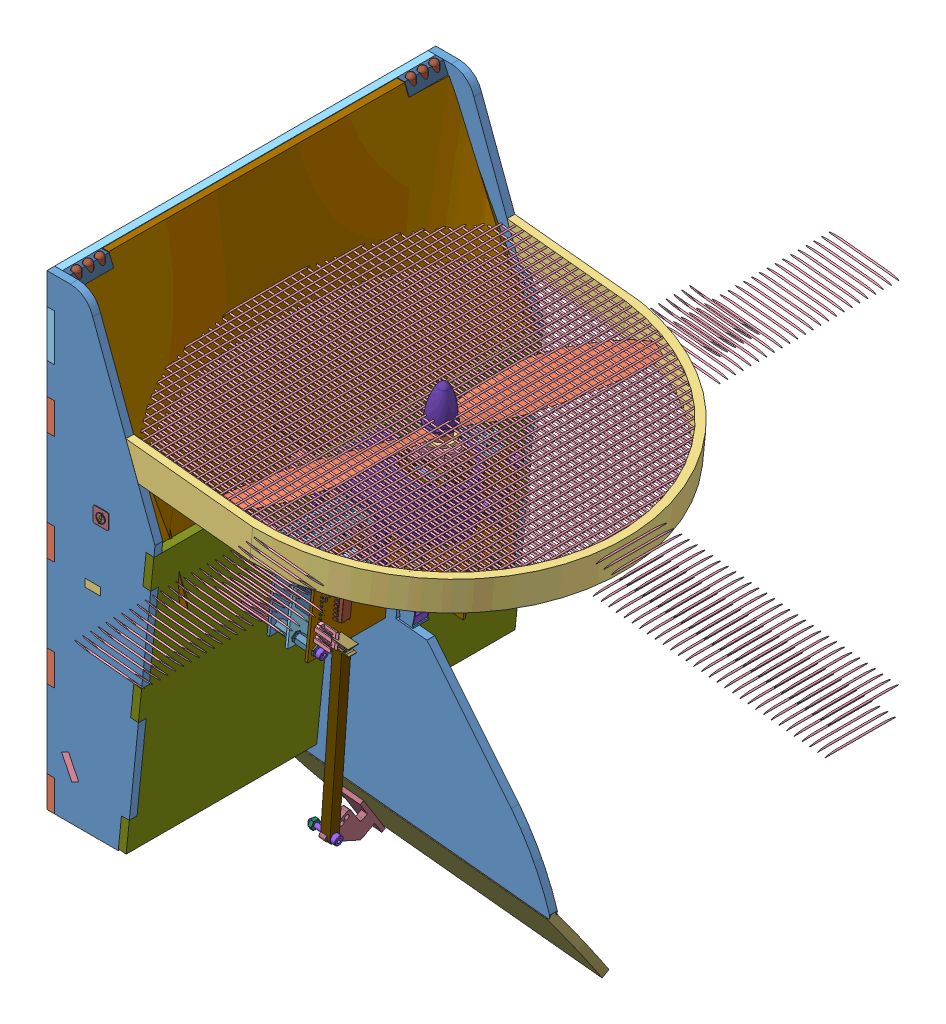
SolidWorks assembly AssTotaleSimu6, configuration Défaut. Lengths in mm. (continued)
Components (placement in the parent): (continued)
- AssStructSimu-1: AssStructSimu [Défaut] at (-125.7658 -1.8483 624.6548) x (1 0 0) z (0 0 -1) size (253.25 324.59 251.6) (continued)
  - AssCarte-1: AssCarte [Défaut] at (38.0121 147.1029 290.772) x (-0.101852 0.9948 0) z (0.9948 0.101852 0) size (66.52 130.57 98.72) (continued)
    - carte_onduleur_v3-1: carte_onduleur_v3 [Défaut] at (-131.8199 12.0892 20.7912) size (66.52 130.57 82.34) (continued)
      - RC2_2-1: RC2_2 [Défaut] at (-22 0.18 -0.803) x (-1 0 0) z (0 0 -1) size (2.34 1.04 0.5) (continued)
        - Open CASCADE STEP translator 6.8 1.12.1-1: Open CASCADE STEP translator 6.8 1.12.1 [Défaut] at origin size (2.34 1.04 0.5) (continued)
          - Pin_2_2-1: Pin_2_2 [Défaut] at origin size (0.51 1.02 0.5)
      - RC3_1-1: RC3_1 [Défaut] at (-20.9336 -14.5 -0.803) x (1 0 0) z (0 0 -1) size (2.34 1.04 0.5)
        - Open CASCADE STEP translator 6.8 1.12.1-1: Open CASCADE STEP translator 6.8 1.12.1 [Défaut] at origin size (2.34 1.04 0.5)
          - Body_1_3-1: Body_1_3 [Défaut] at origin size (2.29 1.04 0.43)
          - Pin_1_2-1: Pin_1_2 [Défaut] at (0.3048 0 0) x (-1 0 0) z (0 0 1) size (0.51 1.02 0.5)
          - Pin_2_2-1: Pin_2_2 [Défaut] at origin size (0.51 1.02 0.5)
      - RC3_2-1: RC3_2 [Défaut] at (-22.3 -14.5 -0.803) x (-1 0 0) z (0 0 -1) size (2.34 1.04 0.5)
        - Open CASCADE STEP translator 6.8 1.12.1-1: Open CASCADE STEP translator 6.8 1.12.1 [Défaut] at origin size (2.34 1.04 0.5)
          - Body_1_3-1: Body_1_3 [Défaut] at origin size (2.29 1.04 0.43)
          - Pin_1_2-1: Pin_1_2 [Défaut] at (0.3048 0 0) x (-1 0 0) z (0 0 1) size (0.51 1.02 0.5)
          - Pin_2_2-1: Pin_2_2 [Défaut] at origin size (0.51 1.02 0.5)
      - U_MES_CUR-1: U_MES_CUR [Défaut] at (-11.5 6.7816 0.803) size (2.54 2.41 0.76)
        - Open CASCADE STEP translator 6.8 1.32.1-1: Open CASCADE STEP translator 6.8 1.32.1 [Défaut] at origin size (2.54 2.41 0.76)
          - Body_1_5-1: Body_1_5 [Défaut] at origin size (2.54 1.27 0.71)
          - Pin_1_3-1: Pin_1_3 [Défaut] at (-2.1082 0.2286 0) x (0 -1 0) z (0 0 1) size (1.14 0.25 0.47)
          - Pin_2_3-1: Pin_2_3 [Défaut] at (-0.2032 2.1336 0) x (0 -1 0) z (0 0 1) size (1.14 0.25 0.47)
      - CARTE_ALIM-1: CARTE_ALIM [Défaut] at (-6.4 -57.2 0.803) size (60 130 18.35)
        - Open CASCADE STEP translator 6.8 1.33.1-1: Open CASCADE STEP translator 6.8 1.33.1 [Défaut] at origin size (60 130 18.35)
          - Body_1_6-1: Body_1_6 [Défaut] at (7 56 -12) size (60 130 18.35)
            - 1_3-1: 1_3 [Défaut] at origin size (60 130 1.61)
            - 13_3-1: 13_3 [Défaut] at (0.4717 -40.93 0.803) x (0 1 0) z (0 0 1) size (5.65 4.9 1.7)
              - =_[0_1_1_4]_3-1: =_[0_1_1_4]_3 [Défaut] at origin size (5.65 4.9 1.7)
                - 2-1: 2 [Défaut] at origin size (3.75 4.9 1.53)
                - 3-1: 3 [Défaut] at origin size (0.95 0.51 1.06)
                - 4-1: 4 [Défaut] at origin size (0.95 0.51 1.06)
                - 5_2-1: 5_2 [Défaut] at origin size (0.95 0.51 1.06)
                - 6-1: 6 [Défaut] at origin size (0.95 0.51 1.06)
                - 7-1: 7 [Défaut] at (10.8 -5.08 0) x (-1 0 0) z (0 0 1) size (0.95 0.51 1.06)
                - 8_2-1: 8_2 [Défaut] at (10.8 -2.54 0) x (-1 0 0) z (0 0 1) size (0.95 0.51 1.06)
                - 9-1: 9 [Défaut] at (10.8 0 0) x (-1 0 0) z (0 0 1) size (0.95 0.51 1.06)
                - 10-1: 10 [Défaut] at (10.8 2.54 0) x (-1 0 0) z (0 0 1) size (0.95 0.51 1.06)
                - 11_2-1: 11_2 [Défaut] at (5.4 -1.27 0) x (-1 0 0) z (0 0 1) size (4.25 2.34 1.06)
            - 18-1: 18 [Défaut] at (-2.5283 -37.23 0.803) x (0 -1 0) z (0 0 1) size (2.34 1.04 0.5)
              - =_[0_1_1_16]-1: =_[0_1_1_16] [Défaut] at origin size (2.34 1.04 0.5)
                - 14_2-1: 14_2 [Défaut] at origin size (2.29 1.04 0.43)
                - 15_2-1: 15_2 [Défaut] at (0.3048 0 0) x (-1 0 0) z (0 0 1) size (0.51 1.02 0.5)
                - 16_2-1: 16_2 [Défaut] at origin size (0.51 1.02 0.5)
            - 21_2-1: 21_2 [Défaut] at (-2.2263 -24.628 -0.803) x (1 0 0) z (0 0 -1) size (8.01 8 14.24)
              - =_[0_1_1_21]-1: =_[0_1_1_21] [Défaut] at origin size (8.01 8 14.24)
                - 19-1: 19 [Défaut] at (1.8 0 0) x (1 0 0) z (0 -1 0) size (8.01 14.24 8)
            - 23_2-1: 23_2 [Défaut] at (1.2381 -31.53 0.803) size (2.34 1.04 0.5)
              - =_[0_1_1_16]-1: =_[0_1_1_16] [Défaut] at origin size (2.34 1.04 0.5)
                - 14_2-1: 14_2 [Défaut] at origin size (2.29 1.04 0.43)
                - 15_2-1: 15_2 [Défaut] at (0.3048 0 0) x (-1 0 0) z (0 0 1) size (0.51 1.02 0.5)
                - 16_2-1: 16_2 [Défaut] at origin size (0.51 1.02 0.5)
            - 28-1: 28 [Défaut] at (5 29.8636 0.803) x (0 -1 0) z (0 0 1) size (3.35 1.3 0.55)
              - =_[0_1_1_25]_2-1: =_[0_1_1_25]_2 [Défaut] at origin size (3.35 1.3 0.55)
                - 24-1: 24 [Défaut] at origin size (3.3 1.3 0.48)
                - 25_2-1: 25_2 [Défaut] at (0.5588 0 0) x (-1 0 0) z (0 0 1) size (0.76 1.27 0.55)
                - 26_2-1: 26_2 [Défaut] at origin size (0.76 1.27 0.55)
            - 30-1: 30 [Défaut] at (6.7 29.8636 0.803) x (0 -1 0) z (0 0 1) size (2.34 1.04 0.5)
              - =_[0_1_1_16]-1: =_[0_1_1_16] [Défaut] at origin size (2.34 1.04 0.5)
                - 14_2-1: 14_2 [Défaut] at origin size (2.29 1.04 0.43)
                - 15_2-1: 15_2 [Défaut] at (0.3048 0 0) x (-1 0 0) z (0 0 1) size (0.51 1.02 0.5)
                - 16_2-1: 16_2 [Défaut] at origin size (0.51 1.02 0.5)
            - 35_2-1: 35_2 [Défaut] at (-2.5 -46.37 0.803) x (0 1 0) z (0 0 1) size (3.4 2.06 0.79)
              - =_[0_1_1_31]-1: =_[0_1_1_31] [Défaut] at origin size (3.4 2.06 0.79)
                - 31_2-1: 31_2 [Défaut] at origin size (3.3 2.06 0.69)
                - 32_3-1: 32_3 [Défaut] at (0.5588 0 0) x (-1 0 0) z (0 0 1) size (0.81 2.03 0.79)
                - 33_3-1: 33_3 [Défaut] at origin size (0.81 2.03 0.79)
            - 37-1: 37 [Défaut] at (5 31.43 0.803) x (0 1 0) z (0 0 1) size (2.34 1.04 0.5)
              - =_[0_1_1_16]-1: =_[0_1_1_16] [Défaut] at origin size (2.34 1.04 0.5)
                - 14_2-1: 14_2 [Défaut] at origin size (2.29 1.04 0.43)
                - 15_2-1: 15_2 [Défaut] at (0.3048 0 0) x (-1 0 0) z (0 0 1) size (0.51 1.02 0.5)
                - 16_2-1: 16_2 [Défaut] at origin size (0.51 1.02 0.5)
            - 39-1: 39 [Défaut] at (-0.2 35.63 0.803) x (-1 0 0) z (0 0 1) size (2.34 1.04 0.5)
              - =_[0_1_1_16]-1: =_[0_1_1_16] [Défaut] at origin size (2.34 1.04 0.5)
                - 14_2-1: 14_2 [Défaut] at origin size (2.29 1.04 0.43)
                - 15_2-1: 15_2 [Défaut] at (0.3048 0 0) x (-1 0 0) z (0 0 1) size (0.51 1.02 0.5)
                - 16_2-1: 16_2 [Défaut] at origin size (0.51 1.02 0.5)
            - 41-1: 41 [Défaut] at (2.9 -45.5036 0.803) x (0 1 0) z (0 0 1) size (2.34 1.04 0.5)
              - =_[0_1_1_16]-1: =_[0_1_1_16] [Défaut] at origin size (2.34 1.04 0.5)
                - 14_2-1: 14_2 [Défaut] at origin size (2.29 1.04 0.43)
                - 15_2-1: 15_2 [Défaut] at (0.3048 0 0) x (-1 0 0) z (0 0 1) size (0.51 1.02 0.5)
                - 16_2-1: 16_2 [Défaut] at origin size (0.51 1.02 0.5)
            - 43-1: 43 [Défaut] at (17.1348 -42.6272 0.803) x (0 1 0) z (0 0 1) size (2.34 1.04 0.5)
              - =_[0_1_1_16]-1: =_[0_1_1_16] [Défaut] at origin size (2.34 1.04 0.5)
                - 14_2-1: 14_2 [Défaut] at origin size (2.29 1.04 0.43)
                - 15_2-1: 15_2 [Défaut] at (0.3048 0 0) x (-1 0 0) z (0 0 1) size (0.51 1.02 0.5)
                - 16_2-1: 16_2 [Défaut] at origin size (0.51 1.02 0.5)
            - 48_2-1: 48_2 [Défaut] at (-5.4717 -39.01 0.803) x (-1 0 0) z (0 0 1) size (4.19 3.4 1.75)
              - =_[0_1_1_40]-1: =_[0_1_1_40] [Défaut] at origin size (4.19 3.4 1.75)
                - 44_2-1: 44_2 [Défaut] at origin size (3.75 3.38 1.73)
                - 45_2-1: 45_2 [Défaut] at (0.438 0 0) x (-1 0 0) z (0 0 1) size (0.53 3.4 1.75)
                - 46_2-1: 46_2 [Défaut] at origin size (0.52 3.4 1.75)
            - 53-1: 53 [Défaut] at (0.9 35.63 0.803) size (2.34 1.04 0.5)
              - =_[0_1_1_45]-1: =_[0_1_1_45] [Défaut] at origin size (2.34 1.04 0.5)
                - 49_3-1: 49_3 [Défaut] at origin size (2.29 1.04 0.43)
                - 50-1: 50 [Défaut] at (0.3048 0 0) x (-1 0 0) z (0 0 1) size (0.51 1.02 0.5)
                - 51-1: 51 [Défaut] at origin size (0.51 1.02 0.5)
            - 55_2-1: 55_2 [Défaut] at (1.3 -45.5036 0.803) x (0 1 0) z (0 0 1) size (2.34 1.04 0.5)
              - =_[0_1_1_45]-1: =_[0_1_1_45] [Défaut] at origin size (2.34 1.04 0.5)
                - 49_3-1: 49_3 [Défaut] at origin size (2.29 1.04 0.43)
                - 50-1: 50 [Défaut] at (0.3048 0 0) x (-1 0 0) z (0 0 1) size (0.51 1.02 0.5)
                - 51-1: 51 [Défaut] at origin size (0.51 1.02 0.5)
            - 57_3-1: 57_3 [Défaut] at (17.2348 -43.9936 0.803) x (0 -1 0) z (0 0 1) size (2.34 1.04 0.5)
              - =_[0_1_1_45]-1: =_[0_1_1_45] [Défaut] at origin size (2.34 1.04 0.5)
                - 49_3-1: 49_3 [Défaut] at origin size (2.29 1.04 0.43)
                - 50-1: 50 [Défaut] at (0.3048 0 0) x (-1 0 0) z (0 0 1) size (0.51 1.02 0.5)
                - 51-1: 51 [Défaut] at origin size (0.51 1.02 0.5)
            - 65-1: 65 [Défaut] at (-4.8 30.93 0.803) x (-1 0 0) z (0 0 1) size (14.64 9.83 4.25)
              - =_[0_1_1_52]-1: =_[0_1_1_52] [Défaut] at origin size (14.64 9.83 4.25)
                - 63_2-1: 63_2 [Défaut] at (3 0 0) x (0 -1 0) z (0 0 1) size (9.83 14.64 4.25)
                  - =_[0_1_1_3]_5-1: =_[0_1_1_3]_5 [Défaut] at origin size (9.83 9.05 4.21)
                  - =_[0_1_1_4]_5-1: =_[0_1_1_4]_5 [Défaut] at origin size (9.48 7.76 1.21)
                  - =_[0_1_1_5]_5-1: =_[0_1_1_5]_5 [Défaut] at origin size (1.36 6.01 3.08)
                  - =_[0_1_1_6]_3-1: =_[0_1_1_6]_3 [Défaut] at origin size (1.36 6.01 3.08)
                  - =_[0_1_1_7]_3-1: =_[0_1_1_7]_3 [Défaut] at origin size (1.06 6.01 3.08)
            - 67-1: 67 [Défaut] at (13.5933 -37.5272 0.803) x (-1 0 0) z (0 0 1) size (2.34 1.04 0.5)
              - =_[0_1_1_16]-1: =_[0_1_1_16] [Défaut] at origin size (2.34 1.04 0.5)
                - 14_2-1: 14_2 [Défaut] at origin size (2.29 1.04 0.43)
                - 15_2-1: 15_2 [Défaut] at (0.3048 0 0) x (-1 0 0) z (0 0 1) size (0.51 1.02 0.5)
                - 16_2-1: 16_2 [Défaut] at origin size (0.51 1.02 0.5)
            - 70_2-1: 70_2 [Défaut] at (18.2733 -29.7272 0.803) x (0 1 0) z (0 0 1) size (6.06 4.95 1.88)
              - =_[0_1_1_61]-1: =_[0_1_1_61] [Défaut] at origin size (6.06 4.95 1.88)
                - 68-1: 68 [Défaut] x (1 0 0) z (0 -1 0) size (6.06 1.88 4.95)
            - 83-1: 83 [Défaut] at (-21.2 -38.07 0.803) x (-1 0 0) z (0 0 1) size (2.7 5.2 1.11)
              - =_[0_1_1_64]-1: =_[0_1_1_64] [Défaut] at origin size (2.7 5.2 1.11)
                - 84_2-1: 84_2 [Défaut] at (1.2 -4 0) x (0 1 0) z (0 0 1) size (5.2 2.7 1.11)
                  - =_[0_1_1_3]_6-1: =_[0_1_1_3]_6 [Défaut] at origin size (0.39 0.64 0.01)
                  - =_[0_1_1_4]_6-1: =_[0_1_1_4]_6 [Défaut] at origin size (0.6 1.9 0.2)
                  - =_[0_1_1_5]_6-1: =_[0_1_1_5]_6 [Défaut] at origin size (0.21 0.08 0.01)
                  - =_[0_1_1_6]_4-1: =_[0_1_1_6]_4 [Défaut] at origin size (0.6 1.9 0.2)
                  - =_[0_1_1_7]_4-1: =_[0_1_1_7]_4 [Défaut] at origin size (0.46 0.68 0.01)
                  - =_[0_1_1_8]_3-1: =_[0_1_1_8]_3 [Défaut] at origin size (0.38 0.66 0.01)
                  - =_[0_1_1_9]_2-1: =_[0_1_1_9]_2 [Défaut] at origin size (0.2 0.62 0.01)
                  - =_[0_1_1_10]_2-1: =_[0_1_1_10]_2 [Défaut] at origin size (4 2.7 1.1)
                  - =_[0_1_1_11]_2-1: =_[0_1_1_11]_2 [Défaut] at origin size (0.46 0.63 0.01)
                  - =_[0_1_1_12]_2-1: =_[0_1_1_12]_2 [Défaut] at origin size (0.56 0.68 0.01)
            - 86_2-1: 86_2 [Défaut] at (12.8933 -35.4272 0.803) x (0 1 0) z (0 0 1) size (2.7 5.2 1.11)
              - =_[0_1_1_77]-1: =_[0_1_1_77] [Défaut] at origin size (2.7 5.2 1.11)
                - 84_2-1: 84_2 [Défaut] at (1.2 -4 0) x (0 1 0) z (0 0 1) size (5.2 2.7 1.11)
                  - =_[0_1_1_3]_6-1: =_[0_1_1_3]_6 [Défaut] at origin size (0.39 0.64 0.01)
                  - =_[0_1_1_4]_6-1: =_[0_1_1_4]_6 [Défaut] at origin size (0.6 1.9 0.2)
                  - =_[0_1_1_5]_6-1: =_[0_1_1_5]_6 [Défaut] at origin size (0.21 0.08 0.01)
                  - =_[0_1_1_6]_4-1: =_[0_1_1_6]_4 [Défaut] at origin size (0.6 1.9 0.2)
                  - =_[0_1_1_7]_4-1: =_[0_1_1_7]_4 [Défaut] at origin size (0.46 0.68 0.01)
                  - =_[0_1_1_8]_3-1: =_[0_1_1_8]_3 [Défaut] at origin size (0.38 0.66 0.01)
                  - =_[0_1_1_9]_2-1: =_[0_1_1_9]_2 [Défaut] at origin size (0.2 0.62 0.01)
                  - =_[0_1_1_10]_2-1: =_[0_1_1_10]_2 [Défaut] at origin size (4 2.7 1.1)
                  - =_[0_1_1_11]_2-1: =_[0_1_1_11]_2 [Défaut] at origin size (0.46 0.63 0.01)
                  - =_[0_1_1_12]_2-1: =_[0_1_1_12]_2 [Défaut] at origin size (0.56 0.68 0.01)
            - 92_2-1: 92_2 [Défaut] at (20.9933 -39.3272 0.803) x (0 -1 0) z (0 0 1) size (2.79 1.98 0.64)
              - =_[0_1_1_79]-1: =_[0_1_1_79] [Défaut] at origin size (2.79 1.98 0.64)
                - 87-1: 87 [Défaut] at origin size (2.79 1.02 0.58)
                - 88-1: 88 [Défaut] x (0 -1 0) z (0 0 1) size (0.42 0.38 0.38)
                - 89-1: 89 [Défaut] at (-2.8448 -0.9652 0) x (0 1 0) z (0 0 1) size (0.55 0.38 0.38)
                - 90-1: 90 [Défaut] at (-0.9652 -2.8448 0) x (0 1 0) z (0 0 1) size (0.55 0.38 0.38)
            - 98-1: 98 [Défaut] at (-17.7 -48.47 0.803) x (0 -1 0) z (0 0 1) size (2.54 1.98 0.64)
              - =_[0_1_1_85]-1: =_[0_1_1_85] [Défaut] at origin size (2.54 1.98 0.64)
                - 93-1: 93 [Défaut] at origin size (2.54 1.14 0.58)
                - 94-1: 94 [Défaut] x (0 -1 0) z (0 0 1) size (0.43 0.51 0.38)
                - 95-1: 95 [Défaut] at (1.8796 1.8796 0) x (0 -1 0) z (0 0 1) size (0.43 0.51 0.38)
                - 96-1: 96 [Défaut] at (-0.9652 -2.8448 0) x (0 1 0) z (0 0 1) size (0.41 0.51 0.38)
            - 100-1: 100 [Défaut] at (24.3933 -43.2272 0.803) size (2.79 1.98 0.64)
              - =_[0_1_1_79]-1: =_[0_1_1_79] [Défaut] at origin size (2.79 1.98 0.64)
                - 87-1: 87 [Défaut] at origin size (2.79 1.02 0.58)
                - 88-1: 88 [Défaut] x (0 -1 0) z (0 0 1) size (0.42 0.38 0.38)
                - 89-1: 89 [Défaut] at (-2.8448 -0.9652 0) x (0 1 0) z (0 0 1) size (0.55 0.38 0.38)
                - 90-1: 90 [Défaut] at (-0.9652 -2.8448 0) x (0 1 0) z (0 0 1) size (0.55 0.38 0.38)
            - 102-1: 102 [Défaut] at (21.4933 -44.4272 0.803) x (0 -1 0) z (0 0 1) size (2.79 1.98 0.64)
              - =_[0_1_1_79]-1: =_[0_1_1_79] [Défaut] at origin size (2.79 1.98 0.64)
                - 87-1: 87 [Défaut] at origin size (2.79 1.02 0.58)
                - 88-1: 88 [Défaut] x (0 -1 0) z (0 0 1) size (0.42 0.38 0.38)
                - 89-1: 89 [Défaut] at (-2.8448 -0.9652 0) x (0 1 0) z (0 0 1) size (0.55 0.38 0.38)
                - 90-1: 90 [Défaut] at (-0.9652 -2.8448 0) x (0 1 0) z (0 0 1) size (0.55 0.38 0.38)
            - 107-1: 107 [Défaut] at (23.1933 -29.1272 -0.803) x (0 1 0) z (0 0 -1) size (9.6 14.35 5)
              - =_[0_1_1_93]-1: =_[0_1_1_93] [Défaut] at origin size (9.6 14.35 5)
                - 105-1: 105 [Défaut] at (0.5 -1 2) x (-1 0 0) z (0 0 1) size (9.6 14.35 5)
                  - =_[0_1_1_3]_7-1: =_[0_1_1_3]_7 [Défaut] at origin size (9.6 12.75 5)
                  - =_[0_1_1_4]_7-1: =_[0_1_1_4]_7 [Défaut] at origin size (2.2 1.6 2.2)
            - 109-1: 109 [Défaut] at (25.4933 -41.1272 0.803) x (-1 0 0) z (0 0 1) size (2.34 1.04 0.5)
              - =_[0_1_1_45]-1: =_[0_1_1_45] [Défaut] at origin size (2.34 1.04 0.5)
                - 49_3-1: 49_3 [Défaut] at origin size (2.29 1.04 0.43)
                - 50-1: 50 [Défaut] at (0.3048 0 0) x (-1 0 0) z (0 0 1) size (0.51 1.02 0.5)
                - 51-1: 51 [Défaut] at origin size (0.51 1.02 0.5)
            - 111-1: 111 [Défaut] at (22.0269 -41.8272 0.803) x (-1 0 0) z (0 0 1) size (2.34 1.04 0.5)
              - =_[0_1_1_45]-1: =_[0_1_1_45] [Défaut] at origin size (2.34 1.04 0.5)
                - 49_3-1: 49_3 [Défaut] at origin size (2.29 1.04 0.43)
                - 50-1: 50 [Défaut] at (0.3048 0 0) x (-1 0 0) z (0 0 1) size (0.51 1.02 0.5)
                - 51-1: 51 [Défaut] at origin size (0.51 1.02 0.5)
            - 113-1: 113 [Défaut] at (-24.8 -36.7036 0.803) x (0 1 0) z (0 0 1) size (2.34 1.04 0.5)
              - =_[0_1_1_45]-1: =_[0_1_1_45] [Défaut] at origin size (2.34 1.04 0.5)
                - 49_3-1: 49_3 [Défaut] at origin size (2.29 1.04 0.43)
                - 50-1: 50 [Défaut] at (0.3048 0 0) x (-1 0 0) z (0 0 1) size (0.51 1.02 0.5)
                - 51-1: 51 [Défaut] at origin size (0.51 1.02 0.5)
            - 115-1: 115 [Défaut] at (-24.8 -40.3036 0.803) x (0 1 0) z (0 0 1) size (2.34 1.04 0.5)
              - =_[0_1_1_45]-1: =_[0_1_1_45] [Défaut] at origin size (2.34 1.04 0.5)
                - 49_3-1: 49_3 [Défaut] at origin size (2.29 1.04 0.43)
                - 50-1: 50 [Défaut] at (0.3048 0 0) x (-1 0 0) z (0 0 1) size (0.51 1.02 0.5)
                - 51-1: 51 [Défaut] at origin size (0.51 1.02 0.5)
            - 117-1: 117 [Défaut] at (-16 -48.27 0.803) x (0 -1 0) z (0 0 1) size (2.34 1.04 0.5)
              - =_[0_1_1_45]-1: =_[0_1_1_45] [Défaut] at origin size (2.34 1.04 0.5)
                - 49_3-1: 49_3 [Défaut] at origin size (2.29 1.04 0.43)
                - 50-1: 50 [Défaut] at (0.3048 0 0) x (-1 0 0) z (0 0 1) size (0.51 1.02 0.5)
                - 51-1: 51 [Défaut] at origin size (0.51 1.02 0.5)
            - 119-1: 119 [Défaut] at (-22.5189 -47.87 0.803) x (-1 0 0) z (0 0 1) size (2.34 1.04 0.5)
              - =_[0_1_1_45]-1: =_[0_1_1_45] [Défaut] at origin size (2.34 1.04 0.5)
                - 49_3-1: 49_3 [Défaut] at origin size (2.29 1.04 0.43)
                - 50-1: 50 [Défaut] at (0.3048 0 0) x (-1 0 0) z (0 0 1) size (0.51 1.02 0.5)
                - 51-1: 51 [Défaut] at origin size (0.51 1.02 0.5)
            - 121-1: 121 [Défaut] at (22.3933 -38.9272 0.803) size (2.34 1.04 0.5)
              - =_[0_1_1_45]-1: =_[0_1_1_45] [Défaut] at origin size (2.34 1.04 0.5)
                - 49_3-1: 49_3 [Défaut] at origin size (2.29 1.04 0.43)
                - 50-1: 50 [Défaut] at (0.3048 0 0) x (-1 0 0) z (0 0 1) size (0.51 1.02 0.5)
                - 51-1: 51 [Défaut] at origin size (0.51 1.02 0.5)
            - 123-1: 123 [Défaut] at (22.0933 -36.4272 0.803) x (-1 0 0) z (0 0 1) size (2.34 1.04 0.5)
              - =_[0_1_1_45]-1: =_[0_1_1_45] [Défaut] at origin size (2.34 1.04 0.5)
                - 49_3-1: 49_3 [Défaut] at origin size (2.29 1.04 0.43)
                - 50-1: 50 [Défaut] at (0.3048 0 0) x (-1 0 0) z (0 0 1) size (0.51 1.02 0.5)
                - 51-1: 51 [Défaut] at origin size (0.51 1.02 0.5)
            - 125-1: 125 [Défaut] at (22.3933 -32.0272 0.803) x (0 -1 0) z (0 0 1) size (2.34 1.04 0.5)
              - =_[0_1_1_45]-1: =_[0_1_1_45] [Défaut] at origin size (2.34 1.04 0.5)
                - 49_3-1: 49_3 [Défaut] at origin size (2.29 1.04 0.43)
                - 50-1: 50 [Défaut] at (0.3048 0 0) x (-1 0 0) z (0 0 1) size (0.51 1.02 0.5)
                - 51-1: 51 [Défaut] at origin size (0.51 1.02 0.5)
            - 127-1: 127 [Défaut] at (17.9597 -23.1272 0.803) size (2.34 1.04 0.5)
              - =_[0_1_1_16]-1: =_[0_1_1_16] [Défaut] at origin size (2.34 1.04 0.5)
                - 14_2-1: 14_2 [Défaut] at origin size (2.29 1.04 0.43)
                - 15_2-1: 15_2 [Défaut] at (0.3048 0 0) x (-1 0 0) z (0 0 1) size (0.51 1.02 0.5)
                - 16_2-1: 16_2 [Défaut] at origin size (0.51 1.02 0.5)
            - 129-1: 129 [Défaut] at (20.0269 -24.9272 0.803) x (-1 0 0) z (0 0 1) size (2.34 1.04 0.5)
              - =_[0_1_1_16]-1: =_[0_1_1_16] [Défaut] at origin size (2.34 1.04 0.5)
                - 14_2-1: 14_2 [Défaut] at origin size (2.29 1.04 0.43)
                - 15_2-1: 15_2 [Défaut] at (0.3048 0 0) x (-1 0 0) z (0 0 1) size (0.51 1.02 0.5)
                - 16_2-1: 16_2 [Défaut] at origin size (0.51 1.02 0.5)
            - 131-1: 131 [Défaut] at (16.9933 -37.5272 0.803) x (-1 0 0) z (0 0 1) size (2.34 1.04 0.5)
              - =_[0_1_1_45]-1: =_[0_1_1_45] [Défaut] at origin size (2.34 1.04 0.5)
                - 49_3-1: 49_3 [Défaut] at origin size (2.29 1.04 0.43)
                - 50-1: 50 [Défaut] at (0.3048 0 0) x (-1 0 0) z (0 0 1) size (0.51 1.02 0.5)
                - 51-1: 51 [Défaut] at origin size (0.51 1.02 0.5)
            - 136-1: 136 [Défaut] at (3.2957 -29.23 0.803) x (-1 0 0) z (0 0 1) size (4.78 2.79 2.03)
              - =_[0_1_1_110]_2-1: =_[0_1_1_110]_2 [Défaut] at origin size (4.78 2.79 2.03)
                - 132-1: 132 [Défaut] at origin size (4.32 2.79 1.78)
                - 133-1: 133 [Défaut] at (0.4572 0 0) x (-1 0 0) z (0 0 1) size (1.02 1.27 1.32)
                - 134-1: 134 [Défaut] at origin size (1.02 1.27 1.32)
            - 141-1: 141 [Défaut] at (0.2436 -33.3673 0.803) size (3.35 1.3 0.55)
              - =_[0_1_1_115]_2-1: =_[0_1_1_115]_2 [Défaut] at origin size (3.35 1.3 0.55)
                - 137-1: 137 [Défaut] at origin size (3.3 1.3 0.48)
                - 138-1: 138 [Défaut] at (0.5588 0 0) x (-1 0 0) z (0 0 1) size (0.76 1.27 0.55)
                - 139-1: 139 [Défaut] at origin size (0.76 1.27 0.55)
            - 143_2-1: 143_2 [Défaut] at (-0.3 -45.47 0.803) x (0 1 0) z (0 0 1) size (2.34 1.04 0.5)
              - =_[0_1_1_16]-1: =_[0_1_1_16] [Défaut] at origin size (2.34 1.04 0.5)
                - 14_2-1: 14_2 [Défaut] at origin size (2.29 1.04 0.43)
                - 15_2-1: 15_2 [Défaut] at (0.3048 0 0) x (-1 0 0) z (0 0 1) size (0.51 1.02 0.5)
                - 16_2-1: 16_2 [Défaut] at origin size (0.51 1.02 0.5)
            - 145-1: 145 [Défaut] at (6.6 31.13 0.803) x (0 1 0) z (0 0 1) size (3.35 1.3 0.55)
              - =_[0_1_1_25]_2-1: =_[0_1_1_25]_2 [Défaut] at origin size (3.35 1.3 0.55)
                - 24-1: 24 [Défaut] at origin size (3.3 1.3 0.48)
                - 25_2-1: 25_2 [Défaut] at (0.5588 0 0) x (-1 0 0) z (0 0 1) size (0.76 1.27 0.55)
                - 26_2-1: 26_2 [Défaut] at origin size (0.76 1.27 0.55)
            - 148-1: 148 [Défaut] at (-7.5 -56.57 0.803) size (15.24 2.54 7.37)
              - =_[0_1_1_122]_2-1: =_[0_1_1_122]_2 [Défaut] at origin size (15.24 2.54 7.37)
                - 146-1: 146 [Défaut] at (6.3 0 1) x (1 0 0) z (0 -1 0) size (15.24 7.37 2.54)
      - COMP1-1: COMP1 [Défaut] at (-16.3 -36.2 0.803) x (-1 0 0) z (0 0 1) size (2.03 1.88 0.51)
        - Open CASCADE STEP translator 6.8 1.34.1-1: Open CASCADE STEP translator 6.8 1.34.1 [Défaut] at origin size (2.03 1.88 0.51)
          - Body_1_6-1: Body_1_6 [Défaut] at origin size (2.03 1.02 0.46)
          - Pin_1_4-1: Pin_1_4 [Défaut] x (0 1 0) z (0 0 1) size (0.45 0.25 0.32)
          - Pin_2_4-1: Pin_2_4 [Défaut] at (0.65 -0.65 0) x (0 1 0) z (0 0 1) size (0.45 0.25 0.32)
          - Pin_3-1: Pin_3 [Défaut] at (1.3 -1.3 0) x (0 1 0) z (0 0 1) size (0.45 0.25 0.32)
          - Pin_4-1: Pin_4 [Défaut] at (-0.5 3.1 0) x (0 -1 0) z (0 0 1) size (0.41 0.25 0.32)
          - Pin_5-1: Pin_5 [Défaut] at (-1.8 1.8 0) x (0 -1 0) z (0 0 1) size (0.41 0.25 0.32)
      - COMP2-1: COMP2 [Défaut] at (-14.3 -9.6 0.803) x (-1 0 0) z (0 0 1) size (2.03 1.88 0.51)
        - Open CASCADE STEP translator 6.8 1.34.1-1: Open CASCADE STEP translator 6.8 1.34.1 [Défaut] at origin size (2.03 1.88 0.51)
          - Body_1_6-1: Body_1_6 [Défaut] at origin size (2.03 1.02 0.46)
          - Pin_1_4-1: Pin_1_4 [Défaut] x (0 1 0) z (0 0 1) size (0.45 0.25 0.32)
          - Pin_2_4-1: Pin_2_4 [Défaut] at (0.65 -0.65 0) x (0 1 0) z (0 0 1) size (0.45 0.25 0.32)
          - Pin_3-1: Pin_3 [Défaut] at (1.3 -1.3 0) x (0 1 0) z (0 0 1) size (0.45 0.25 0.32)
          - Pin_4-1: Pin_4 [Défaut] at (-0.5 3.1 0) x (0 -1 0) z (0 0 1) size (0.41 0.25 0.32)
          - Pin_5-1: Pin_5 [Défaut] at (-1.8 1.8 0) x (0 -1 0) z (0 0 1) size (0.41 0.25 0.32)
      - COMP3-1: COMP3 [Défaut] at (-15.9 -23.2 0.803) x (-1 0 0) z (0 0 1) size (2.03 1.88 0.51)
        - Open CASCADE STEP translator 6.8 1.34.1-1: Open CASCADE STEP translator 6.8 1.34.1 [Défaut] at origin size (2.03 1.88 0.51)
          - Body_1_6-1: Body_1_6 [Défaut] at origin size (2.03 1.02 0.46)
          - Pin_1_4-1: Pin_1_4 [Défaut] x (0 1 0) z (0 0 1) size (0.45 0.25 0.32)
          - Pin_2_4-1: Pin_2_4 [Défaut] at (0.65 -0.65 0) x (0 1 0) z (0 0 1) size (0.45 0.25 0.32)
          - Pin_3-1: Pin_3 [Défaut] at (1.3 -1.3 0) x (0 1 0) z (0 0 1) size (0.45 0.25 0.32)
          - Pin_4-1: Pin_4 [Défaut] at (-0.5 3.1 0) x (0 -1 0) z (0 0 1) size (0.41 0.25 0.32)
          - Pin_5-1: Pin_5 [Défaut] at (-1.8 1.8 0) x (0 -1 0) z (0 0 1) size (0.41 0.25 0.32)
      - CP1-1: CP1 [Défaut] at (-18.9 -38.2 0.803) x (0 1 0) z (0 0 1) size (2.34 1.04 0.5)
        - Open CASCADE STEP translator 6.8 1.6.1-1: Open CASCADE STEP translator 6.8 1.6.1 [Défaut] at origin size (2.34 1.04 0.5)
          - Body_1-1: Body_1 [Défaut] at origin size (2.29 1.04 0.43)
          - Pin_1-1: Pin_1 [Défaut] at (0.3048 0 0) x (-1 0 0) z (0 0 1) size (0.51 1.02 0.5)
          - Pin_2-1: Pin_2 [Défaut] at origin size (0.51 1.02 0.5)
      - CP2-1: CP2 [Défaut] at (-16.9 -11.6 0.803) x (0 1 0) z (0 0 1) size (2.34 1.04 0.5)
        - Open CASCADE STEP translator 6.8 1.6.1-1: Open CASCADE STEP translator 6.8 1.6.1 [Défaut] at origin size (2.34 1.04 0.5)
          - Body_1-1: Body_1 [Défaut] at origin size (2.29 1.04 0.43)
          - Pin_1-1: Pin_1 [Défaut] at (0.3048 0 0) x (-1 0 0) z (0 0 1) size (0.51 1.02 0.5)
          - Pin_2-1: Pin_2 [Défaut] at origin size (0.51 1.02 0.5)
      - CP3-1: CP3 [Défaut] at (-18.5 -25.2 0.803) x (0 1 0) z (0 0 1) size (2.34 1.04 0.5)
        - Open CASCADE STEP translator 6.8 1.6.1-1: Open CASCADE STEP translator 6.8 1.6.1 [Défaut] at origin size (2.34 1.04 0.5)
          - Body_1-1: Body_1 [Défaut] at origin size (2.29 1.04 0.43)
          - Pin_1-1: Pin_1 [Défaut] at (0.3048 0 0) x (-1 0 0) z (0 0 1) size (0.51 1.02 0.5)
          - Pin_2-1: Pin_2 [Défaut] at origin size (0.51 1.02 0.5)
      - C_DEC_COM1-1: C_DEC_COM1 [Défaut] at (-15 -36 0.803) x (0 -1 0) z (0 0 1) size (2.34 1.04 0.5)
        - Open CASCADE STEP translator 6.8 1.6.1-1: Open CASCADE STEP translator 6.8 1.6.1 [Défaut] at origin size (2.34 1.04 0.5)
          - Body_1-1: Body_1 [Défaut] at origin size (2.29 1.04 0.43)
          - Pin_1-1: Pin_1 [Défaut] at (0.3048 0 0) x (-1 0 0) z (0 0 1) size (0.51 1.02 0.5)
          - Pin_2-1: Pin_2 [Défaut] at origin size (0.51 1.02 0.5)
      - C_DEC_COMP2-1: C_DEC_COMP2 [Défaut] at (-13 -9.3 0.803) x (0 -1 0) z (0 0 1) size (2.34 1.04 0.5)
        - Open CASCADE STEP translator 6.8 1.6.1-1: Open CASCADE STEP translator 6.8 1.6.1 [Défaut] at origin size (2.34 1.04 0.5)
          - Body_1-1: Body_1 [Défaut] at origin size (2.29 1.04 0.43)
          - Pin_1-1: Pin_1 [Défaut] at (0.3048 0 0) x (-1 0 0) z (0 0 1) size (0.51 1.02 0.5)
          - Pin_2-1: Pin_2 [Défaut] at origin size (0.51 1.02 0.5)
      - C_DEC_COMP3-1: C_DEC_COMP3 [Défaut] at (-14.6 -22.9 0.803) x (0 -1 0) z (0 0 1) size (2.34 1.04 0.5)
        - Open CASCADE STEP translator 6.8 1.6.1-1: Open CASCADE STEP translator 6.8 1.6.1 [Défaut] at origin size (2.34 1.04 0.5)
          - Body_1-1: Body_1 [Défaut] at origin size (2.29 1.04 0.43)
          - Pin_1-1: Pin_1 [Défaut] at (0.3048 0 0) x (-1 0 0) z (0 0 1) size (0.51 1.02 0.5)
          - Pin_2-1: Pin_2 [Défaut] at origin size (0.51 1.02 0.5)
      - D_VBAT-1: D_VBAT [Défaut] at (-1.2 46.4 0.803) x (0 -1 0) z (0 0 1) size (2.34 1.04 0.5)
        - Open CASCADE STEP translator 6.8 1.6.1-1: Open CASCADE STEP translator 6.8 1.6.1 [Défaut] at origin size (2.34 1.04 0.5)
          - Body_1-1: Body_1 [Défaut] at origin size (2.29 1.04 0.43)
          - Pin_1-1: Pin_1 [Défaut] at (0.3048 0 0) x (-1 0 0) z (0 0 1) size (0.51 1.02 0.5)
          - Pin_2-1: Pin_2 [Défaut] at origin size (0.51 1.02 0.5)
      - D_3V-1: D_3V [Défaut] at (1.3 46.3 0.803) x (0 -1 0) z (0 0 1) size (2.34 1.04 0.5)
        - Open CASCADE STEP translator 6.8 1.6.1-1: Open CASCADE STEP translator 6.8 1.6.1 [Défaut] at origin size (2.34 1.04 0.5)
          - Body_1-1: Body_1 [Défaut] at origin size (2.29 1.04 0.43)
          - Pin_1-1: Pin_1 [Défaut] at (0.3048 0 0) x (-1 0 0) z (0 0 1) size (0.51 1.02 0.5)
          - Pin_2-1: Pin_2 [Défaut] at origin size (0.51 1.02 0.5)
      - D_5V-1: D_5V [Défaut] at (-3.7 46.4 0.803) x (0 -1 0) z (0 0 1) size (2.34 1.04 0.5)
        - Open CASCADE STEP translator 6.8 1.6.1-1: Open CASCADE STEP translator 6.8 1.6.1 [Défaut] at origin size (2.34 1.04 0.5)
          - Body_1-1: Body_1 [Défaut] at origin size (2.29 1.04 0.43)
          - Pin_1-1: Pin_1 [Défaut] at (0.3048 0 0) x (-1 0 0) z (0 0 1) size (0.51 1.02 0.5)
          - Pin_2-1: Pin_2 [Défaut] at origin size (0.51 1.02 0.5)
      - R1_1-1: R1_1 [Défaut] at (-20.2 -36.1 0.803) x (-1 0 0) z (0 0 1) size (2.34 1.04 0.5)
        - Open CASCADE STEP translator 6.8 1.12.1-1: Open CASCADE STEP translator 6.8 1.12.1 [Défaut] at origin size (2.34 1.04 0.5)
          - Body_1_3-1: Body_1_3 [Défaut] at origin size (2.29 1.04 0.43)
          - Pin_1_2-1: Pin_1_2 [Défaut] at (0.3048 0 0) x (-1 0 0) z (0 0 1) size (0.51 1.02 0.5)
          - Pin_2_2-1: Pin_2_2 [Défaut] at origin size (0.51 1.02 0.5)
      - R1_2-1: R1_2 [Défaut] at (-15.5 -34.6 0.803) x (-1 0 0) z (0 0 1) size (2.34 1.04 0.5)
        - Open CASCADE STEP translator 6.8 1.12.1-1: Open CASCADE STEP translator 6.8 1.12.1 [Défaut] at origin size (2.34 1.04 0.5)
          - Body_1_3-1: Body_1_3 [Défaut] at origin size (2.29 1.04 0.43)
          - Pin_1_2-1: Pin_1_2 [Défaut] at (0.3048 0 0) x (-1 0 0) z (0 0 1) size (0.51 1.02 0.5)
          - Pin_2_2-1: Pin_2_2 [Défaut] at origin size (0.51 1.02 0.5)
      - R1_3-1: R1_3 [Défaut] at (-20.3 -39.9 0.803) x (-1 0 0) z (0 0 1) size (2.34 1.04 0.5)
        - Open CASCADE STEP translator 6.8 1.12.1-1: Open CASCADE STEP translator 6.8 1.12.1 [Défaut] at origin size (2.34 1.04 0.5)
          - Body_1_3-1: Body_1_3 [Défaut] at origin size (2.29 1.04 0.43)
          - Pin_1_2-1: Pin_1_2 [Défaut] at (0.3048 0 0) x (-1 0 0) z (0 0 1) size (0.51 1.02 0.5)
          - Pin_2_2-1: Pin_2_2 [Défaut] at origin size (0.51 1.02 0.5)
      - R1_4-1: R1_4 [Défaut] at (-20.3 -38.1 0.803) x (-1 0 0) z (0 0 1) size (2.34 1.04 0.5)
        - Open CASCADE STEP translator 6.8 1.12.1-1: Open CASCADE STEP translator 6.8 1.12.1 [Défaut] at origin size (2.34 1.04 0.5)
          - Body_1_3-1: Body_1_3 [Défaut] at origin size (2.29 1.04 0.43)
          - Pin_1_2-1: Pin_1_2 [Défaut] at (0.3048 0 0) x (-1 0 0) z (0 0 1) size (0.51 1.02 0.5)
          - Pin_2_2-1: Pin_2_2 [Défaut] at origin size (0.51 1.02 0.5)
      - R1_5-1: R1_5 [Défaut] at (-17.1336 -39.7 0.803) size (2.34 1.04 0.5)
        - Open CASCADE STEP translator 6.8 1.12.1-1: Open CASCADE STEP translator 6.8 1.12.1 [Défaut] at origin size (2.34 1.04 0.5)
          - Body_1_3-1: Body_1_3 [Défaut] at origin size (2.29 1.04 0.43)
          - Pin_1_2-1: Pin_1_2 [Défaut] at (0.3048 0 0) x (-1 0 0) z (0 0 1) size (0.51 1.02 0.5)
          - Pin_2_2-1: Pin_2_2 [Défaut] at origin size (0.51 1.02 0.5)
      - R2_1-1: R2_1 [Défaut] at (-18.5 -9.5 0.803) x (-1 0 0) z (0 0 1) size (2.34 1.04 0.5)
        - Open CASCADE STEP translator 6.8 1.12.1-1: Open CASCADE STEP translator 6.8 1.12.1 [Défaut] at origin size (2.34 1.04 0.5)
          - Body_1_3-1: Body_1_3 [Défaut] at origin size (2.29 1.04 0.43)
          - Pin_1_2-1: Pin_1_2 [Défaut] at (0.3048 0 0) x (-1 0 0) z (0 0 1) size (0.51 1.02 0.5)
          - Pin_2_2-1: Pin_2_2 [Défaut] at origin size (0.51 1.02 0.5)
      - R2_2-1: R2_2 [Défaut] at (-13.1 -8 0.803) x (-1 0 0) z (0 0 1) size (2.34 1.04 0.5)
        - Open CASCADE STEP translator 6.8 1.12.1-1: Open CASCADE STEP translator 6.8 1.12.1 [Défaut] at origin size (2.34 1.04 0.5)
          - Body_1_3-1: Body_1_3 [Défaut] at origin size (2.29 1.04 0.43)
          - Pin_1_2-1: Pin_1_2 [Défaut] at (0.3048 0 0) x (-1 0 0) z (0 0 1) size (0.51 1.02 0.5)
          - Pin_2_2-1: Pin_2_2 [Défaut] at origin size (0.51 1.02 0.5)
      - R2_3-1: R2_3 [Défaut] at (-18.5 -11.2 0.803) x (-1 0 0) z (0 0 1) size (2.34 1.04 0.5)
        - Open CASCADE STEP translator 6.8 1.12.1-1: Open CASCADE STEP translator 6.8 1.12.1 [Défaut] at origin size (2.34 1.04 0.5)
          - Body_1_3-1: Body_1_3 [Défaut] at origin size (2.29 1.04 0.43)
          - Pin_1_2-1: Pin_1_2 [Défaut] at (0.3048 0 0) x (-1 0 0) z (0 0 1) size (0.51 1.02 0.5)
          - Pin_2_2-1: Pin_2_2 [Défaut] at origin size (0.51 1.02 0.5)
      - R2_4-1: R2_4 [Défaut] at (-18.5 -12.8 0.803) x (-1 0 0) z (0 0 1) size (2.34 1.04 0.5)
        - Open CASCADE STEP translator 6.8 1.12.1-1: Open CASCADE STEP translator 6.8 1.12.1 [Défaut] at origin size (2.34 1.04 0.5)
          - Body_1_3-1: Body_1_3 [Défaut] at origin size (2.29 1.04 0.43)
          - Pin_1_2-1: Pin_1_2 [Défaut] at (0.3048 0 0) x (-1 0 0) z (0 0 1) size (0.51 1.02 0.5)
          - Pin_2_2-1: Pin_2_2 [Défaut] at origin size (0.51 1.02 0.5)
      - R2_5-1: R2_5 [Défaut] at (-15.1336 -13 0.803) size (2.34 1.04 0.5)
        - Open CASCADE STEP translator 6.8 1.12.1-1: Open CASCADE STEP translator 6.8 1.12.1 [Défaut] at origin size (2.34 1.04 0.5)
          - Body_1_3-1: Body_1_3 [Défaut] at origin size (2.29 1.04 0.43)
          - Pin_1_2-1: Pin_1_2 [Défaut] at (0.3048 0 0) x (-1 0 0) z (0 0 1) size (0.51 1.02 0.5)
          - Pin_2_2-1: Pin_2_2 [Défaut] at origin size (0.51 1.02 0.5)
      - R3_1-1: R3_1 [Défaut] at (-19.9 -23.1 0.803) x (-1 0 0) z (0 0 1) size (2.34 1.04 0.5)
        - Open CASCADE STEP translator 6.8 1.12.1-1: Open CASCADE STEP translator 6.8 1.12.1 [Défaut] at origin size (2.34 1.04 0.5)
          - Body_1_3-1: Body_1_3 [Défaut] at origin size (2.29 1.04 0.43)
          - Pin_1_2-1: Pin_1_2 [Défaut] at (0.3048 0 0) x (-1 0 0) z (0 0 1) size (0.51 1.02 0.5)
          - Pin_2_2-1: Pin_2_2 [Défaut] at origin size (0.51 1.02 0.5)
      - R3_2-1: R3_2 [Défaut] at (-14.7 -21.6 0.803) x (-1 0 0) z (0 0 1) size (2.34 1.04 0.5)
        - Open CASCADE STEP translator 6.8 1.12.1-1: Open CASCADE STEP translator 6.8 1.12.1 [Défaut] at origin size (2.34 1.04 0.5)
          - Body_1_3-1: Body_1_3 [Défaut] at origin size (2.29 1.04 0.43)
          - Pin_1_2-1: Pin_1_2 [Défaut] at (0.3048 0 0) x (-1 0 0) z (0 0 1) size (0.51 1.02 0.5)
          - Pin_2_2-1: Pin_2_2 [Défaut] at origin size (0.51 1.02 0.5)
      - R3_3-1: R3_3 [Défaut] at (-19.9 -24.8 0.803) x (-1 0 0) z (0 0 1) size (2.34 1.04 0.5)
        - Open CASCADE STEP translator 6.8 1.12.1-1: Open CASCADE STEP translator 6.8 1.12.1 [Défaut] at origin size (2.34 1.04 0.5)
          - Body_1_3-1: Body_1_3 [Défaut] at origin size (2.29 1.04 0.43)
          - Pin_1_2-1: Pin_1_2 [Défaut] at (0.3048 0 0) x (-1 0 0) z (0 0 1) size (0.51 1.02 0.5)
          - Pin_2_2-1: Pin_2_2 [Défaut] at origin size (0.51 1.02 0.5)
      - R3_4-1: R3_4 [Défaut] at (-19.9 -26.4 0.803) x (-1 0 0) z (0 0 1) size (2.34 1.04 0.5)
        - Open CASCADE STEP translator 6.8 1.12.1-1: Open CASCADE STEP translator 6.8 1.12.1 [Défaut] at origin size (2.34 1.04 0.5)
          - Body_1_3-1: Body_1_3 [Défaut] at origin size (2.29 1.04 0.43)
          - Pin_1_2-1: Pin_1_2 [Défaut] at (0.3048 0 0) x (-1 0 0) z (0 0 1) size (0.51 1.02 0.5)
          - Pin_2_2-1: Pin_2_2 [Défaut] at origin size (0.51 1.02 0.5)
      - R3_5-1: R3_5 [Défaut] at (-16.7336 -26.5 0.803) size (2.34 1.04 0.5)
        - Open CASCADE STEP translator 6.8 1.12.1-1: Open CASCADE STEP translator 6.8 1.12.1 [Défaut] at origin size (2.34 1.04 0.5)
          - Body_1_3-1: Body_1_3 [Défaut] at origin size (2.29 1.04 0.43)
          - Pin_1_2-1: Pin_1_2 [Défaut] at (0.3048 0 0) x (-1 0 0) z (0 0 1) size (0.51 1.02 0.5)
          - Pin_2_2-1: Pin_2_2 [Défaut] at origin size (0.51 1.02 0.5)
      - R_LED_3V3-1: R_LED_3V3 [Défaut] at (1.3 47.9 0.803) x (0 1 0) z (0 0 1) size (2.34 1.04 0.5)
        - Open CASCADE STEP translator 6.8 1.12.1-1: Open CASCADE STEP translator 6.8 1.12.1 [Défaut] at origin size (2.34 1.04 0.5)
          - Body_1_3-1: Body_1_3 [Défaut] at origin size (2.29 1.04 0.43)
          - Pin_1_2-1: Pin_1_2 [Défaut] at (0.3048 0 0) x (-1 0 0) z (0 0 1) size (0.51 1.02 0.5)
          - Pin_2_2-1: Pin_2_2 [Défaut] at origin size (0.51 1.02 0.5)
      - R_LED_5V-1: R_LED_5V [Défaut] at (-3.7 47.7 0.803) x (0 1 0) z (0 0 1) size (2.34 1.04 0.5)
        - Open CASCADE STEP translator 6.8 1.12.1-1: Open CASCADE STEP translator 6.8 1.12.1 [Défaut] at origin size (2.34 1.04 0.5)
          - Body_1_3-1: Body_1_3 [Défaut] at origin size (2.29 1.04 0.43)
          - Pin_1_2-1: Pin_1_2 [Défaut] at (0.3048 0 0) x (-1 0 0) z (0 0 1) size (0.51 1.02 0.5)
          - Pin_2_2-1: Pin_2_2 [Défaut] at origin size (0.51 1.02 0.5)
      - R_LED_VBAT-1: R_LED_VBAT [Défaut] at (-1.2 47.9 0.803) x (0 1 0) z (0 0 1) size (2.34 1.04 0.5)
        - Open CASCADE STEP translator 6.8 1.12.1-1: Open CASCADE STEP translator 6.8 1.12.1 [Défaut] at origin size (2.34 1.04 0.5)
          - Body_1_3-1: Body_1_3 [Défaut] at origin size (2.29 1.04 0.43)
          - Pin_1_2-1: Pin_1_2 [Défaut] at (0.3048 0 0) x (-1 0 0) z (0 0 1) size (0.51 1.02 0.5)
          - Pin_2_2-1: Pin_2_2 [Défaut] at origin size (0.51 1.02 0.5)
    - AssEntretoise-1: AssEntretoise [Défaut] at (-156.8199 -51.2976 37.1344) x (0 0 -1) z (1 0 0) size (58.24 7.29 7.81)
      - socket head cap screw 4762_din-1: socket head cap screw 4762_din [EN ISO 4762 M3 x 5 - 5N] at (-2.4967 0.5867 0) size (8 5.5 5.5)
      - hexagonal_spacer_MF_M3_H20_HEX5.5_FTD6_MTL6-1: hexagonal_spacer_MF_M3_H20_HEX5.5_FTD6_MTL6 [Défaut] at (48.3433 0.5867 0) x (0 0 1) z (-1 0 0) size (6.36 5.51 26)
      - hex nut style 1 gradeab_din-1: hex nut style 1 gradeab_din [Hexagon Nut ISO 4032 - M3 - W - N] at (53.3433 0.5867 0) x (0 0.943962 0.330053) z (-1 0 0) size (5.5 6.35 2.4)
      - hexagonal_spacer_MF_M3_H12_HEX5.5_FTD6_MTL6-2: hexagonal_spacer_MF_M3_H12_HEX5.5_FTD6_MTL6 [Défaut] at (27.0633 0.5867 0) x (0 0.248308 0.968681) z (-1 0 0) size (6.36 5.51 18)
      - hexagonal_spacer_MF_M3_H12_HEX5.5_FTD6_MTL6-3: hexagonal_spacer_MF_M3_H12_HEX5.5_FTD6_MTL6 [Défaut] at (13.7833 0.5867 0) x (0 0 1) z (-1 0 0) size (6.36 5.51 18)
    - AssEntretoise-2: AssEntretoise [Défaut] at (-156.8199 68.7024 37.1344) x (0 0 -1) z (1 0 0) size (58.24 7.29 7.81)
      - socket head cap screw 4762_din-1: socket head cap screw 4762_din [EN ISO 4762 M3 x 5 - 5N] at (-2.4967 0.5867 0) size (8 5.5 5.5)
      - hexagonal_spacer_MF_M3_H20_HEX5.5_FTD6_MTL6-1: hexagonal_spacer_MF_M3_H20_HEX5.5_FTD6_MTL6 [Défaut] at (48.3433 0.5867 0) x (0 0 1) z (-1 0 0) size (6.36 5.51 26)
      - hex nut style 1 gradeab_din-1: hex nut style 1 gradeab_din [Hexagon Nut ISO 4032 - M3 - W - N] at (53.3433 0.5867 0) x (0 0.943962 0.330053) z (-1 0 0) size (5.5 6.35 2.4)
      - hexagonal_spacer_MF_M3_H12_HEX5.5_FTD6_MTL6-2: hexagonal_spacer_MF_M3_H12_HEX5.5_FTD6_MTL6 [Défaut] at (27.0633 0.5867 0) x (0 0.248308 0.968681) z (-1 0 0) size (6.36 5.51 18)
      - hexagonal_spacer_MF_M3_H12_HEX5.5_FTD6_MTL6-3: hexagonal_spacer_MF_M3_H12_HEX5.5_FTD6_MTL6 [Défaut] at (13.7833 0.5867 0) x (0 0 1) z (-1 0 0) size (6.36 5.51 18)
